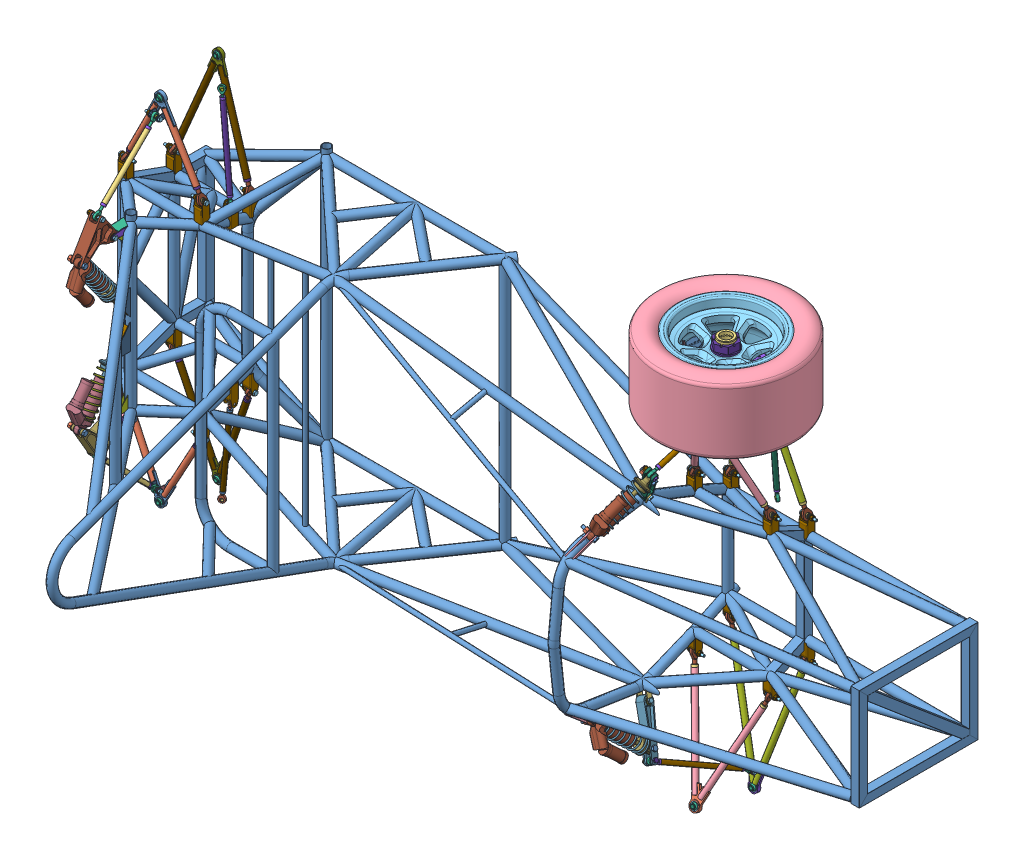
SolidWorks assembly AE-Rolling Chassis Assembly, configuration Default. Lengths in mm. (continued)
Components (placement in the parent): (continued)
- WT-A0100-AH-Corner Assembly-1: WT-A0100-AH-Corner Assembly [Front Left Corner Assembly] at (231.003 -38.1001 -73.813) x (1 0 0) z (0 0 1) size (411.48 213.5 411.48)
  - WT-00202-AA-Hoosier R25B 16x7_5-10-1: WT-00202-AA-Hoosier R25B 16x7_5-10 [Default] at (794.064 613.0884 197.9453) x (0 0 -1) z (0 -1 0) size (411.48 411.48 213.5)
  - WT-00201-AA-OZ Centerlock 10in Wheel-1: WT-00201-AA-OZ Centerlock 10in Wheel [Default] at (794.064 635.0884 197.9453) x (0.604277 0 -0.796774) z (0 1 0) size (288.79 288.79 189.86)
  - WT-####-AB-Misuni Drive Pins-24: WT-####-AB-Misuni Drive Pins [Default] at (833.7507 623.0884 202.9426) x (0 1 0) z (-0.363068 0 0.931762) size (21.1 11.95 11.95)
  - BR-FL20602-AC-Brake Hat-3: BR-FL20602-AC-Brake Hat [Default] at (794.0641 608.9576 197.9453) x (-0.604276 0 0.796775) z (-0.796775 0 -0.604276) size (120.29 4.76 113.7)
  - BR-20601-AA-Brake Rotor-2: BR-20601-AA-Brake Rotor [Default] at (794.0641 608.9576 197.9453) x (-0.992165 0 -0.124931) z (0.124931 0 -0.992165) size (190.5 4.76 190.5)
  - CP4227-2S0-2: CP4227-2S0 [Default] at (809.9391 608.9576 197.9254) x (0.998694 0 0.051087) z (-0.051087 0 0.998694) size (71.54 66.42 130.94)
    - CP4227-2S0.STEP-1: CP4227-2S0.STEP [Default] x (0 0 -1) z (0 -1 0) size (130.94 71.54 66.42)
      - CP4227-101.STEP-1: CP4227-101.STEP [Default] at origin size (112 60.5 34.68)
      - CP4227-102.STEP-1: CP4227-102.STEP [Default] x (-1 0 0) z (0 0 -1) size (109 47.57 30.98)
      - cp3049-40a_CP4226-103.STEP-1: cp3049-40a_CP4226-103.STEP [Default] at (-23.4668 -94.12 -10.305) size (25.2 25.2 14.87)
      - cp3049-40a_CP4226-103.STEP-2: cp3049-40a_CP4226-103.STEP [Default] at (-23.4668 -94.12 10.305) x (-0.98369 0.179874 0) z (0 0 -1) size (25.2 25.2 14.87)
      - cp3049-40a_CP4226-103.STEP-3: cp3049-40a_CP4226-103.STEP [Default] at (23.4668 -94.12 10.305) x (-0.960147 0.279495 0) z (0 0 -1) size (25.2 25.2 14.87)
      - cp3049-40a_CP4226-103.STEP-4: cp3049-40a_CP4226-103.STEP [Default] at (23.4668 -94.12 -10.305) size (25.2 25.2 14.87)
      - cp3838-M08x1.25m_CP4477-110.STEP-1: cp3838-M08x1.25m_CP4477-110.STEP [Default] at (-41.1 -109.6 19.55) x (-0.998897 0.046962 0) z (0 0 -1) size (13 13 46)
      - cp3838-M08x1.25m_CP4477-110.STEP-2: cp3838-M08x1.25m_CP4477-110.STEP [Default] at (0 -116.83 19.55) x (-0.99038 0.138378 0) z (0 0 -1) size (13 13 46)
      - cp3838-M08x1.25m_CP4477-110.STEP-3: cp3838-M08x1.25m_CP4477-110.STEP [Default] at (41.1 -109.6 19.55) x (-1 -0.000032 0) z (0 0 -1) size (13 13 46)
      - cp4226-104_CP4226-104.STEP-1: cp4226-104_CP4226-104.STEP [Default] at (-29.0318 -116.44 -31.75) x (0 0 1) z (1 0 0) size (61.35 20.1 3)
      - cp4226-104_CP4226-104.STEP-2: cp4226-104_CP4226-104.STEP [Default] at (29.0318 -116.44 -31.75) x (0 0 1) z (1 0 0) size (61.35 20.1 3)
      - CP4469-101.STEP-1: CP4469-101.STEP [Default] at (-65.47 -82.62 -23.98) x (0 0.474307 -0.88036) z (1 0 0) size (9.24 8.21 29.15)
      - CP4469-101.STEP-2: CP4469-101.STEP [Default] at (65.47 -82.62 -23.98) x (0 0.509894 0.860237) z (-1 0 0) size (9.24 8.21 29.15)
      - CP4226-4m.STEP-1: CP4226-4m.STEP [Default] at (10.0433 -40.2815 10.305) x (0.970296 0.241922 0) z (0 0 -1) size (39.7 43.64 7)
      - CP4226-4m.STEP-2: CP4226-4m.STEP [Default] at (10.0433 -40.2815 -10.305) x (-0.970296 -0.241922 0) z (0 0 1) size (39.7 43.64 7)
      - CP4226-4m.STEP-3: CP4226-4m.STEP [Default] at (-10.0433 -40.2815 -10.305) x (-0.970296 0.241922 0) z (0 0 1) size (39.7 43.64 7)
      - CP4226-4m.STEP-4: CP4226-4m.STEP [Default] at (-10.0433 -40.2815 10.305) x (0.970296 -0.241922 0) z (0 0 -1) size (39.7 43.64 7)
  - WT-20104-AC-Sensor Ring-2: WT-20104-AC-Sensor Ring [Default] at (794.0641 606.5764 197.9453) x (-0.992165 0 -0.124931) z (0 -1 0) size (113.66 114.3 1.59)
  - WT-10102-AA-Centerlock Nut-2: WT-10102-AA-Centerlock Nut [Default] at (794.064 685.7079 197.9453) x (-0.796775 0 -0.604276) z (0.604276 0 -0.796775) size (66 31.75 66)
  - WT-AA-Camber Block-2: WT-AA-Camber Block [Default] at (789.2314 585.9914 292.4205) x (-0.998694 0 -0.051087) z (-0.048552 -0.311078 0.949143) size (47.63 44.45 33.35)
  - WT-AF-Upright-1: WT-AF-Upright [Default] at (794.0641 576.6365 197.9453) x (-0.998694 0 -0.051087) z (-0.051087 0 0.998694) size (101.76 54.5 217.79)
  - 1985-1932-TheTimkenCompany-3D-01-05-2023.stp-1: 1985-1932-TheTimkenCompany-3D-01-05-2023.stp [Default] at (794.0641 573.7663 197.9453) x (0 -1 0) z (0.770726 0 0.637167) size (21.39 58.74 58.74)
  - WT-10101-AB-Wheel Hub Front-1: WT-10101-AB-Wheel Hub Front [Front] at (794.0641 623.6579 197.9453) x (0.992165 0 0.124931) z (-0.124931 0 0.992165) size (96.32 138.68 96.32)
  - 1985-1932-TheTimkenCompany-3D-01-05-2023.stp-2: 1985-1932-TheTimkenCompany-3D-01-05-2023.stp [Default] at (794.0641 579.5067 197.9453) x (0 1 0) z (0.64822 0 -0.761453) size (21.39 58.74 58.74)
  - WT-10106-AB-Backing Plate-1: WT-10106-AB-Backing Plate [Default] at (794.0641 554.4115 197.9453) x (0.757216 0 -0.653165) z (0.653165 0 0.757216) size (57.91 5.08 57.91)
  - WT-AA- Front Grease Seal-2: WT-AA- Front Grease Seal [Default] at (794.0641 601.5556 197.9453) x (-0.615562 0 -0.788088) z (-0.788088 0 0.615562) size (58.42 7.71 58.42)
  - WT-A8###-AA-Front Toe Bracket-1: WT-A8###-AA-Front Toe Bracket [Default] at (814.3917 551.9812 107.1998) x (0.998694 0 0.051087) z (-0.051087 0 0.998694) size (40.8 37.93 55.25)
    - WT-FB-Toe Base Plate-1: WT-FB-Toe Base Plate [Default] at (22.5935 33.4208 28.102) size (3.17 37.93 55.25)
    - WT-FB-Toe Bottom Clevis-1: WT-FB-Toe Bottom Clevis [Default] at (-402.1509 50.6365 13.751) size (40.8 37.86 3.17)
    - WT-FB-Toe Top Clevis-1: WT-FB-Toe Top Clevis [Default] at (52.058 56.7183 39.278) size (40.8 37.86 3.17)
  - BR-FR20603-AA-Floating Bobbins-1: BR-FR20603-AA-Floating Bobbins [Default] at (853.9165 609.1322 205.4818) x (1 0 0) z (0 0 1) size (12.7 8.29 12.7)
  - BR-FR20603-AA-Floating Bobbins-2: BR-FR20603-AA-Floating Bobbins [Default] at (817.4635 609.1322 253.5472) x (0.5 0 0.866025) z (-0.866025 0 0.5) size (12.7 8.29 12.7)
  - BR-FR20603-AA-Floating Bobbins-3: BR-FR20603-AA-Floating Bobbins [Default] at (757.6111 609.1322 246.0108) x (-0.5 0 0.866025) z (-0.866025 0 -0.5) size (12.7 8.29 12.7)
  - BR-FR20603-AA-Floating Bobbins-4: BR-FR20603-AA-Floating Bobbins [Default] at (734.2117 609.1323 190.4089) x (-1 0 0) z (0 0 -1) size (12.7 8.29 12.7)
  - BR-FR20603-AA-Floating Bobbins-5: BR-FR20603-AA-Floating Bobbins [Default] at (770.6647 609.1323 142.3434) x (-0.5 0 -0.866025) z (0.866025 0 -0.5) size (12.7 8.29 12.7)
  - BR-FR20603-AA-Floating Bobbins-6: BR-FR20603-AA-Floating Bobbins [Default] at (830.517 609.1323 149.8799) x (0.5 0 -0.866025) z (0.866025 0 0.5) size (12.7 8.29 12.7)
  - WT-####-AB-Misuni Drive Pins-28: WT-####-AB-Misuni Drive Pins [Default] at (789.0668 623.0884 237.6319) x (0 1 0) z (-0.931762 0 -0.363068) size (21.1 11.95 11.95)
  - WT-####-AB-Misuni Drive Pins-29: WT-####-AB-Misuni Drive Pins [Default] at (754.3775 623.0884 192.948) x (0 1 0) z (0.363068 0 -0.931762) size (21.1 11.95 11.95)
  - WT-####-AB-Misuni Drive Pins-30: WT-####-AB-Misuni Drive Pins [Default] at (799.0614 623.0884 158.2588) x (0 1 0) z (0.931762 0 0.363068) size (21.1 11.95 11.95)
  - 97447A110_Aluminum Blind Rivets with Aluminum Mandrel-1: 97447A110_Aluminum Blind Rivets with Aluminum Mandrel [97447A110] at (835.6457 604.9889 203.1812) x (0.907339 0 0.4204) z (0 -1 0) size (5.03 5.03 11.56)
  - 97447A110_Aluminum Blind Rivets with Aluminum Mandrel-6: 97447A110_Aluminum Blind Rivets with Aluminum Mandrel [97447A110] at (810.3205 604.9889 236.574) x (0.089592 0 0.995979) z (0 -1 0) size (5.03 5.03 11.56)
  - 97447A110_Aluminum Blind Rivets with Aluminum Mandrel-5: 97447A110_Aluminum Blind Rivets with Aluminum Mandrel [97447A110] at (768.7389 604.9889 231.3382) x (-0.817747 0 0.575578) z (0 -1 0) size (5.03 5.03 11.56)
  - 97447A110_Aluminum Blind Rivets with Aluminum Mandrel-4: 97447A110_Aluminum Blind Rivets with Aluminum Mandrel [97447A110] at (752.4824 604.9889 192.7095) x (-0.907339 0 -0.4204) z (0 -1 0) size (5.03 5.03 11.56)
  - 97447A110_Aluminum Blind Rivets with Aluminum Mandrel-3: 97447A110_Aluminum Blind Rivets with Aluminum Mandrel [97447A110] at (777.8076 604.9889 159.3166) x (-0.089592 0 -0.995979) z (0 -1 0) size (5.03 5.03 11.56)
  - 97447A110_Aluminum Blind Rivets with Aluminum Mandrel-2: 97447A110_Aluminum Blind Rivets with Aluminum Mandrel [97447A110] at (819.3893 604.9889 164.5525) x (0.817747 0 -0.575578) z (0 -1 0) size (5.03 5.03 11.56)
  - 93070A181_Alloy Steel Low-Profile Socket Head Screw-1: 93070A181_Alloy Steel Low-Profile Socket Head Screw [93070A181] at (740.9846 579.1176 146.3354) x (0 -1 0) z (0 0 1) size (45.29 13 13)
  - 93070A181_Alloy Steel Low-Profile Socket Head Screw-2: 93070A181_Alloy Steel Low-Profile Socket Head Screw [93070A181] at (736.0803 579.1176 242.2101) x (0 -1 0) z (0 0 1) size (45.29 13 13)
  - FS-Jet Nut, M8x1.25 (MJET-M8X1.25)-1: FS-Jet Nut, M8x1.25 (MJET-M8X1.25) [Default] at (736.0803 582.4576 242.2101) x (0.837169 0 0.546944) z (0 -1 0) size (13.6 13.6 7)
  - FS-Jet Nut, M8x1.25 (MJET-M8X1.25)-2: FS-Jet Nut, M8x1.25 (MJET-M8X1.25) [Default] at (740.9846 582.4576 146.3354) x (-0.837169 0 -0.546944) z (0 -1 0) size (13.6 13.6 7)
  - 91251A350_Black-Oxide Alloy Steel Socket Head Screw-1: 91251A350_Black-Oxide Alloy Steel Socket Head Screw [91251A350] at (834.2542 574.2103 161.7878) x (0.049303 0.261936 -0.963825) z (0.998694 0 0.051087) size (7.94 7.94 16.01)
  - 91251A350_Black-Oxide Alloy Steel Socket Head Screw-4: 91251A350_Black-Oxide Alloy Steel Socket Head Screw [91251A350] at (835.4866 589.9176 136.4176) x (0.049303 0.261936 -0.963825) z (0.998694 0 0.051087) size (7.94 7.94 16.01)
  - 91251A350_Black-Oxide Alloy Steel Socket Head Screw-2: 91251A350_Black-Oxide Alloy Steel Socket Head Screw [91251A350] at (834.1891 593.0926 161.7844) x (0.049303 0.261936 -0.963825) z (0.998694 0 0.051087) size (7.94 7.94 16.01)
  - 91290A442_Alloy Steel Socket Head Screw-1: 91290A442_Alloy Steel Socket Head Screw [91290A442] at (801.7277 597.1822 296.7274) x (0.912214 -0.113442 0.393696) z (0.015892 -0.950384 -0.310672) size (13 13 48.09)
  - 91290A442_Alloy Steel Socket Head Screw-2: 91290A442_Alloy Steel Socket Head Screw [91290A442] at (776.3608 597.1822 295.4298) x (-0.912214 0.113442 -0.393696) z (0.015892 -0.950384 -0.310672) size (13 13 48.09)
  - FS-Jet Nut, M8x1.25 (MJET-M8X1.25)-3: FS-Jet Nut, M8x1.25 (MJET-M8X1.25) [Default] at (776.3966 595.0438 294.7308) x (0.999807 0.011523 0.015892) z (-0.015892 0.950384 0.310672) size (13.6 13.6 7)
  - FS-Jet Nut, M8x1.25 (MJET-M8X1.25)-4: FS-Jet Nut, M8x1.25 (MJET-M8X1.25) [Default] at (801.7634 595.0438 296.0284) x (0.543038 -0.252689 0.800786) z (-0.015892 0.950384 0.310672) size (13.6 13.6 7) (hidden)
  - 3528N13_High-Strength Steel Distorted-Thread Flange Locknut-1: 3528N13_High-Strength Steel Distorted-Thread Flange Locknut [3528N13] at (794.0641 619.8329 197.9453) x (-0.585494 0 -0.810677) z (0 1 0) size (21.8 21.8 11.4)
  - 98093A648_Black-Phosphate Class 10.9 Steel Screw-2: 98093A648_Black-Phosphate Class 10.9 Steel Screw [98093A648] at (794.0641 589.1315 197.9453) x (-0.837171 0 -0.546942) z (0 -1 0) size (22.3 22.3 100.4)
- WT-A0100-XG-Corner Assembly-1: WT-A0100-XG-Corner Assembly [Front Left Corner Assembly] at (222.4405 0 -72.1526) size (411.48 213.6 411.53) (hidden)
  - WT-RL00202-AA-Hoosier R25B 16x7_5-10-1: WT-RL00202-AA-Hoosier R25B 16x7_5-10 [Default] at (-793.1174 574.9879 198.909) x (-1 0 0) z (0 -1 0.000253) size (411.48 411.48 213.5)
  - WT-RL00201-AA-OZ Centerlock 10in Wheel-1: WT-RL00201-AA-OZ Centerlock 10in Wheel [Default] at (-793.1174 596.9879 198.9034) x (-0.992442 0.000031 0.122714) z (0 1 -0.000253) size (288.79 288.79 189.86)
  - WT-RL####-AB-Misuni Drive Pins-8: WT-RL####-AB-Misuni Drive Pins [Default] at (-825.0424 584.994 223.0062) x (0 1 -0.000253) z (0.897414 0.000112 0.44119) size (21.1 11.95 11.95)
  - WT-RL10102-AA-Centerlock Nut-1: WT-RL10102-AA-Centerlock Nut [Default] at (-793.1174 647.6073 198.8906) x (0.34363 0.000238 0.939105) z (-0.939105 0.000087 0.34363) size (66 31.75 66)
  - WT-RL####-XF-Upright-1: WT-RL####-XF-Upright [Default] at (-793.1174 537.8923 198.9183) x (-0.999961 -0.000002 -0.008824) z (-0.008824 0.000253 0.999961) size (134.42 50.23 211.08)
  - BR-A0102-AA-Caliper Assembly-1: BR-A0102-AA-Caliper Assembly [Default] at (-874.0145 570.8565 194.5235) x (-0.069854 0.000252 0.997557) z (0 -1 0.000253) size (40.11 43.54 52.73)
    - cp3838-M08x1.25m_CP4477-110^BR-A0102-AA-Caliper Assembly-1: cp3838-M08x1.25m_CP4477-110^BR-A0102-AA-Caliper Assembly [Default] at (-13.37 19.3 19.55) x (-0.999952 -0.009843 0) z (0 0 -1) size (13 13 46) (virtual)
    - CP4226-102^BR-A0102-AA-Caliper Assembly-1: CP4226-102^BR-A0102-AA-Caliper Assembly [Default] x (-1 0 0) z (0 0 -1) size (63.87 47.42 31.57) (virtual)
    - cp4226-104_CP4226-104^BR-A0102-AA-Caliper Assembly-1: cp4226-104_CP4226-104^BR-A0102-AA-Caliper Assembly [Default] at (0 23 -31.9644) x (0 0 1) z (-1 0 0) size (61.35 20.1 3) (virtual)
    - CP4226-101^BR-A0102-AA-Caliper Assembly-1: CP4226-101^BR-A0102-AA-Caliper Assembly [Default] at origin size (81.26 55.69 34.68) (virtual)
    - cp3838-M08x1.25m_CP4477-110^BR-A0102-AA-Caliper Assembly-2: cp3838-M08x1.25m_CP4477-110^BR-A0102-AA-Caliper Assembly [Default] at (13.37 19.3 19.55) x (-0.997666 -0.068288 0) z (0 0 -1) size (13 13 46) (virtual)
    - cp3049-40a_CP4226-103^BR-A0102-AA-Caliper Assembly-1: cp3049-40a_CP4226-103^BR-A0102-AA-Caliper Assembly [Default] at (0 0 10.305) x (-0.993137 0.116957 0) z (0 0 -1) size (25.2 25.2 14.87) (virtual)
    - CP4469-101^BR-A0102-AA-Caliper Assembly-1: CP4469-101^BR-A0102-AA-Caliper Assembly [Default] at (42 -11.5 -23.98) x (0 -0.520643 0.853775) z (-1 0 0) size (9.18 8.2 29.15) (virtual)
    - cp3049-40a_CP4226-103^BR-A0102-AA-Caliper Assembly-2: cp3049-40a_CP4226-103^BR-A0102-AA-Caliper Assembly [Default] at (0 0 -10.305) size (25.2 25.2 14.87) (virtual)
    - Brake Pad^BR-A0102-AA-Caliper Assembly-1: Brake Pad^BR-A0102-AA-Caliper Assembly [Default] at (0 11.1798 8.5855) x (-1 0 0) z (0 -1 0) size (39.62 6.86 43.54) (virtual)
    - Brake Pad^BR-A0102-AA-Caliper Assembly-2: Brake Pad^BR-A0102-AA-Caliper Assembly [Default] at (0 11.1798 -8.5905) x (1 0 0) z (0 -1 0) size (39.62 6.86 43.54) (virtual)
  - WT-RL10103-AA-Grease Seal-1: WT-RL10103-AA-Grease Seal [Default] at (-793.1174 559.091 198.913) x (-0.781145 -0.000158 -0.624349) z (-0.624349 0.000198 0.781145) size (97.66 13.92 97.66)
  - LL713049-LL713010-TheTimkenCompany-3D-11-03-2022.stp-1: LL713049-LL713010-TheTimkenCompany-3D-11-03-2022.stp [Default] at (-793.1174 541.0673 198.9175) x (0 1 -0.000253) z (0.586717 -0.000205 -0.809792) size (15.53 98.42 98.42)
  - LL713049-LL713010-TheTimkenCompany-3D-11-03-2022.stp-2: LL713049-LL713010-TheTimkenCompany-3D-11-03-2022.stp [Default] at (-793.1174 534.7173 198.9191) x (0 -1 0.000253) z (0.531557 -0.000214 -0.847022) size (15.53 98.42 98.42)
  - WT-XA-Tripod Nut-1: WT-XA-Tripod Nut [Default] at (-793.1174 516.4598 198.9238) x (0 1 -0.000253) z (0.798123 -0.000152 -0.602494) size (30.44 98.37 98.37)
  - WT-RL####-BA-Camber Block-1: WT-RL####-BA-Camber Block [Default] at (-793.95 547.3609 293.2547) x (-0.999961 -0.000002 -0.008824) z (-0.008819 -0.034647 0.999361) size (82.61 35.93 35.38)
  - 91290A442_Alloy Steel Socket Head Screw-1: 91290A442_Alloy Steel Socket Head Screw [91290A442] at (-816.177 556.8302 293.3869) x (0.914102 0.014329 -0.405231) z (0.000308 -0.9994 -0.034645) size (13 13 48.09)
  - BR-A0000-AB-Rear Brake Assembly-1: BR-A0000-AB-Rear Brake Assembly [Default No Bobbins] at (-793.1174 596.9879 198.9034) x (-0.602494 -0.000202 -0.798123) z (-0.798123 0.000152 0.602494) size (251.55 172.72 251.55)
    - WT-XA-#####-Tripod Hub-2: WT-XA-#####-Tripod Hub [Default] at origin size (102.86 172.72 102.86)
    - BR-20601-AB-Brake Rotor-1: BR-20601-AB-Brake Rotor [Default] at (0 26.1303 0) x (0.866025 0 -0.5) z (0.5 0 0.866025) size (184.15 4.76 184.15)
    - BR-20603-BA-Floating Bobbins-1: BR-20603-BA-Floating Bobbins [Default] at (39.8696 25.9874 23.0188) size (15.88 8.92 15.88)
    - BR-20603-BA-Floating Bobbins-2: BR-20603-BA-Floating Bobbins [Default] at (0 25.9874 46.0375) x (0.5 0 0.866025) z (-0.866025 0 0.5) size (15.88 8.92 15.88)
    - BR-20603-BA-Floating Bobbins-3: BR-20603-BA-Floating Bobbins [Default] at (-39.8696 25.9874 23.0188) x (-0.5 0 0.866025) z (-0.866025 0 -0.5) size (15.88 8.92 15.88)
    - BR-20603-BA-Floating Bobbins-4: BR-20603-BA-Floating Bobbins [Default] at (-39.8696 25.9874 -23.0188) x (-1 0 0) z (0 0 -1) size (15.88 8.92 15.88)
    - BR-20603-BA-Floating Bobbins-5: BR-20603-BA-Floating Bobbins [Default] at (0 25.9874 -46.0375) x (-0.5 0 -0.866025) z (0.866025 0 -0.5) size (15.88 8.92 15.88)
    - BR-20603-BA-Floating Bobbins-6: BR-20603-BA-Floating Bobbins [Default] at (39.8696 25.9874 -23.0188) x (0.5 0 -0.866025) z (0.866025 0 0.5) size (15.88 8.92 15.88)
    - WT-20104-AB-Rear Sensor Ring-1: WT-20104-AB-Rear Sensor Ring [Default] at (0 30.099 0) x (0.882948 0 -0.469472) z (0 -1 0) size (137 137 1.59)
    - 91590A121_External Retaining Ring-1: 91590A121_External Retaining Ring [91590A121] at (-39.8696 29.2354 23.0188) x (0 1 0) z (-0.857167 0 0.515038) size (0.64 14.63 13.25)
    - 91590A121_External Retaining Ring-2: 91590A121_External Retaining Ring [91590A121] at (-39.8696 29.2354 -23.0188) x (0 1 0) z (-0.87462 0 -0.48481) size (0.64 14.63 13.25)
    - 91590A121_External Retaining Ring-3: 91590A121_External Retaining Ring [91590A121] at (0 29.2354 -46.0375) x (0 1 0) z (-0.017452 0 -0.999848) size (0.64 14.63 13.25)
    - 91590A121_External Retaining Ring-4: 91590A121_External Retaining Ring [91590A121] at (39.8696 29.2354 -23.0188) x (0 1 0) z (0.857167 0 -0.515038) size (0.64 14.63 13.25)
    - 91590A121_External Retaining Ring-5: 91590A121_External Retaining Ring [91590A121] at (39.8696 29.2354 23.0188) x (0 1 0) z (0.87462 0 0.48481) size (0.64 14.63 13.25)
    - 91590A121_External Retaining Ring-6: 91590A121_External Retaining Ring [91590A121] at (0 29.2354 46.0375) x (0 1 0) z (0.017452 0 0.999848) size (0.64 14.63 13.25)
    - 97447A110_Aluminum Blind Rivets with Aluminum Mandrel-1: 97447A110_Aluminum Blind Rivets with Aluminum Mandrel [97447A110] at (9.6137 30.099 51.8707) x (-0.302097 0 -0.953277) z (0 1 0) size (5.03 5.03 11.56)
    - 97447A110_Aluminum Blind Rivets with Aluminum Mandrel-2: 97447A110_Aluminum Blind Rivets with Aluminum Mandrel [97447A110] at (-40.1145 30.099 34.261) x (0.674514 0 -0.738262) z (0 1 0) size (5.03 5.03 11.56)
    - 97447A110_Aluminum Blind Rivets with Aluminum Mandrel-3: 97447A110_Aluminum Blind Rivets with Aluminum Mandrel [97447A110] at (-49.7282 30.099 -17.6097) x (0.976611 0 0.215015) z (0 1 0) size (5.03 5.03 11.56)
    - 97447A110_Aluminum Blind Rivets with Aluminum Mandrel-4: 97447A110_Aluminum Blind Rivets with Aluminum Mandrel [97447A110] at (-9.6137 30.099 -51.8707) x (0.302097 0 0.953277) z (0 1 0) size (5.03 5.03 11.56)
    - 97447A110_Aluminum Blind Rivets with Aluminum Mandrel-5: 97447A110_Aluminum Blind Rivets with Aluminum Mandrel [97447A110] at (40.1145 30.099 -34.261) x (-0.674514 0 0.738262) z (0 1 0) size (5.03 5.03 11.56)
    - 97447A110_Aluminum Blind Rivets with Aluminum Mandrel-6: 97447A110_Aluminum Blind Rivets with Aluminum Mandrel [97447A110] at (49.7282 30.099 17.6097) x (-0.976611 0 -0.215015) z (0 1 0) size (5.03 5.03 11.56)
  - FS-Jet Nut, M8x1.25 (MJET-M8X1.25)-1: FS-Jet Nut, M8x1.25 (MJET-M8X1.25) [Default] at (-816.1783 561.0546 293.5333) x (-0.906747 0.01433 -0.421432) z (-0.000308 0.9994 0.034645) size (13.6 13.6 7)
  - 91290A442_Alloy Steel Socket Head Screw-2: 91290A442_Alloy Steel Socket Head Screw [91290A442] at (-771.7287 556.8303 293.7791) x (-0.549228 0.028783 -0.835176) z (0.000308 -0.9994 -0.034645) size (13 13 48.09)
  - FS-Jet Nut, M8x1.25 (MJET-M8X1.25)-2: FS-Jet Nut, M8x1.25 (MJET-M8X1.25) [Default] at (-771.73 561.0547 293.9256) x (0.139109 0.034351 -0.989681) z (-0.000308 0.9994 0.034645) size (13.6 13.6 7)
  - WT-RL####-AB-Misuni Drive Pins-21: WT-RL####-AB-Misuni Drive Pins [Default] at (-769.0177 584.9959 230.8313) x (0 1 -0.000253) z (0.44119 -0.000227 -0.897414) size (21.1 11.95 11.95)
  - WT-RL####-AB-Misuni Drive Pins-22: WT-RL####-AB-Misuni Drive Pins [Default] at (-761.1925 584.9818 174.8066) x (0 1 -0.000253) z (-0.897414 -0.000112 -0.44119) size (21.1 11.95 11.95)
  - WT-RL####-AB-Misuni Drive Pins-23: WT-RL####-AB-Misuni Drive Pins [Default] at (-817.2172 584.9798 166.9815) x (0 1 -0.000253) z (-0.44119 0.000227 0.897414) size (21.1 11.95 11.95)
  - WT-AA-#####-Rear Toe Backing Plate-1: WT-AA-#####-Rear Toe Backing Plate [Default] at (-737.4958 539.7904 186.7082) x (0.999961 0.000002 0.008824) z (-0.008824 0.000253 0.999961) size (3.17 25.4 50.8)
  - WT-AA-#####-Rear Toe Top Clevis-1: WT-AA-#####-Rear Toe Top Clevis [Default] at (-737.5965 542.9683 198.1116) x (0.999961 0.000002 0.008824) z (-0.008824 0.000253 0.999961) size (31.75 27.83 3.17)
  - WT-AA-#####-Rear Toe Bottom Clevis-1: WT-AA-#####-Rear Toe Bottom Clevis [Default] at (-737.3694 539.7868 172.3832) x (0.999961 0.000002 0.008824) z (-0.008824 0.000253 0.999961) size (31.75 27.12 3.17)
  - 91251A350_Black-Oxide Alloy Steel Socket Head Screw-1: 91251A350_Black-Oxide Alloy Steel Socket Head Screw [91251A350] at (-737.6322 543.6053 205.7568) x (0.008824 -0.000002 -0.999961) z (0.999961 0.000002 0.008824) size (7.94 7.94 16.01)
  - 91251A350_Black-Oxide Alloy Steel Socket Head Screw-2: 91251A350_Black-Oxide Alloy Steel Socket Head Screw [91251A350] at (-737.4641 533.4404 186.7101) x (0.008809 0.059166 -0.998209) z (0.999961 0.000002 0.008824) size (7.94 7.94 16.01)
  - 91251A350_Black-Oxide Alloy Steel Socket Head Screw-3: 91251A350_Black-Oxide Alloy Steel Socket Head Screw [91251A350] at (-737.4641 546.1404 186.7069) x (0.008824 -0.000002 -0.999961) z (0.999961 0.000002 0.008824) size (7.94 7.94 16.01)
Mates (geometry in assembly coordinates):
- Coincident1: coordinate: point of FR-A0100-FG_3-Space_Frame-1
- Coincident2: coincident: point of FR-A0100-FG_3-Space_Frame-1; point of SP-A0200-AD-Front Axle Assembly-1
- Coincident3: coincident: point of FR-A0100-FG_3-Space_Frame-1; point of SP-A0200-AD-Front Axle Assembly-1
- Coincident4: coincident: point of FR-A0100-FG_3-Space_Frame-1; point of SP-A0200-AD-Front Axle Assembly-1
- Coincident5: coincident: point of FR-A0100-FG_3-Space_Frame-1; point of SP-A0200-AI-Rear Axle Assembly-1
- Coincident6: coincident: point of FR-A0100-FG_3-Space_Frame-1; point of SP-A0200-AI-Rear Axle Assembly-1
- Parallel1: parallel aligned: plane of SP-A0200-AI-Rear Axle Assembly-1 through (222.4405 0 -72.1526) normal (0 0 1)
- Coincident9: coincident: point of SP-A0200-AD-Front Axle Assembly-1; point of WT-A0100-AH-Corner Assembly-1
- Coincident10: coincident aligned: line of SP-A0200-AD-Front Axle Assembly-1 through (231.003 -38.1001 -73.813) axis (0 1 0); line of WT-A0100-AH-Corner Assembly-1 through (231.003 -38.1001 -73.813) axis (0 1 0)
- Coincident11: coincident aligned: line of SP-A0200-AD-Front Axle Assembly-1 through (231.003 -38.1001 -73.813) axis (1 0 0); line of WT-A0100-AH-Corner Assembly-1 through (231.003 -38.1001 -73.813) axis (1 0 0)
- Coincident12: coincident: point of SP-A0200-AI-Rear Axle Assembly-1; point of WT-A0100-XG-Corner Assembly-1
- Coincident13: coincident aligned: line of SP-A0200-AI-Rear Axle Assembly-1 through (-571.5 0 -72.1526) axis (0 1 0); line of WT-A0100-XG-Corner Assembly-1 through (-571.5 0 -72.1526) axis (0 1 0)
